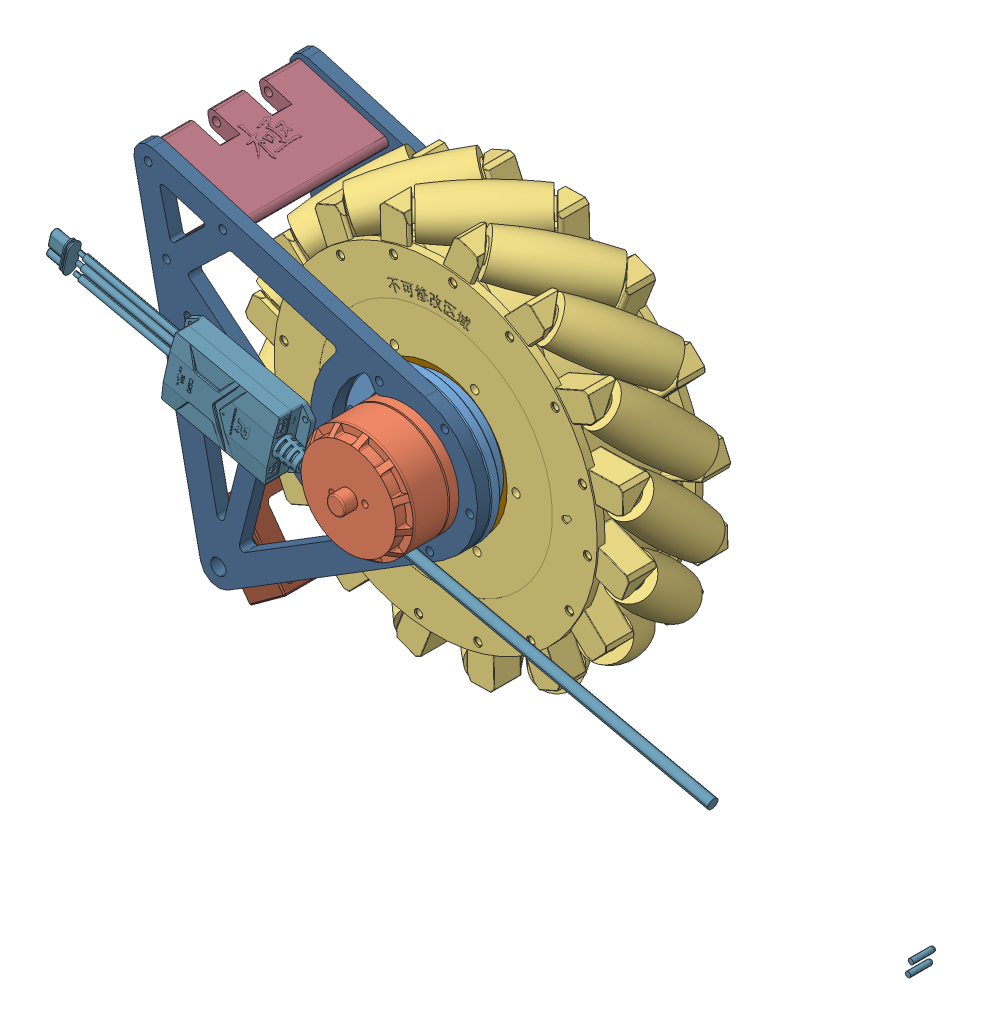
SolidWorks assembly 轮组2, configuration 默认. Lengths in mm.
Overall size (340.98 169.14 98.4).
20 component instances, 16 part files, 46 mates.
Components (placement in the parent):
- 轮组3508机加工件-1: 轮组3508机加工件 [默认] x (-0.923728 -0.383049 0) z (0 0 -1) size (56.5 56.5 41)
- RM3508直流无刷减速电机-1: RM3508直流无刷减速电机 [默认] at (-14.2303 -11.5943 46.941) x (-0.704187 0.710014 0) z (0 0 -1) size (42 44.97 98.4)
- HEXROLL_16-D154-2.0-1: HEXROLL_16-D154-2.0 [默认] at (0 0 -7.05) x (0.999858 0.01686 0) z (0 0 1) size (153.78 153.78 41)
- 轮组转动机加件-1: 轮组转动机加件 [默认] at (0 0 -42.1) x (0 0 -1) z (0.857472 0.51453 0) size (22 67 67)
- 轮组机加件-1: 轮组机加件 [默认] at (0 0 -18) x (0 0 1) z (0.01686 -0.999858 0) size (8 66 66)
- 胀紧套 ZZ21—10x20x13-1: 胀紧套 ZZ21—10x20x13 [默认] at (0 0 -47.8) x (-0.281461 -0.959573 0) z (0 0 -1) size (20 20 15.5)
- GB894．2-86轴用弹性挡圈B型25-1: GB894．2-86轴用弹性挡圈B型25 [默认] at (0 0 -62.2) x (-0.199141 -0.979971 0) z (0 0 1) size (28.2 30.93 1.2)
- 法兰轴承-1: 法兰轴承 [25*37*7-1.5] at (0 0 -61.6) x (0.478869 0.877886 0) z (0.877886 -0.478869 0) size (40 7 40)
- 深沟球轴承-1: 深沟球轴承 [45x58x7] at (0 0 -17) x (0.721643 -0.692266 0) z (-0.692266 -0.721643 0) size (58 7 58)
- 轮组转板-1: 轮组转板 [内侧板] at (-98.9523 52.4637 2.5) x (-0.97621 -0.216826 0) z (0 0 -1) size (120.47 137.51 5)
- 轮组转板-2: 轮组转板 [外侧板] at (-98.9523 52.4637 -57.6) x (-0.97621 -0.216826 0) z (0 0 -1) size (120.47 137.51 5)
- 轮组转点机加工件-1: 轮组转点机加工件 [默认] at (-71.8517 -69.551 -27.55) x (0 0 1) z (-0.808472 -0.588535 0) size (45 30 17)
- 轮组垫块-1: 轮组垫块 [默认] at (0 0 -61.6) x (0.97621 0.216826 0) z (0 0 1) size (56.5 56.5 1.5)
- 悬挂安装打印件-1: 悬挂安装打印件 [默认] at (-98.9523 52.4637 -27.6) x (0.722068 0.691822 0) z (0 0 1) size (37.46 32.98 55)
- C620无刷电机调速器-2: C620无刷电机调速器 [默认] at (-61.9578 -5.1134 10.4) x (-0.976343 0.216228 0) z (-0.216228 -0.976343 0) size (343.45 13.81 26.13)
- 深沟球轴承-2: 深沟球轴承 [6x13x5] at (-71.8517 -69.551 -50.05) x (-0.458973 -0.88845 0) z (-0.88845 0.458973 0) size (13 5 13)
- 深沟球轴承-3: 深沟球轴承 [6x13x5] at (-71.8517 -69.551 -10.05) x (0.999149 0.04124 0) z (0.04124 -0.999149 0) size (13 5 13)
- 推力球轴承-1: 推力球轴承 [F6-14M 6*14*5] at (-71.8517 -69.551 -5.05) x (-0.205581 -0.97864 0) z (-0.97864 0.205581 0) size (14 5 14)
- 推力球轴承-2: 推力球轴承 [F6-14M 6*14*5] at (-71.8517 -69.551 -55.05) x (0.195364 -0.980731 0) z (-0.980731 -0.195364 0) size (14 5 14)
- 轮组轴承压板-1: 轮组轴承压板 [默认] at (0 0 -63.6) x (0.97621 0.216826 0) z (0 0 1) size (56.5 56.5 2)
Mates (geometry in assembly coordinates):
- 同心1: concentric aligned: cylinder of 轮组3508机加工件-1 through (0 0 -4) axis (0 0 1) radius 28.25; cylinder of 轮组转板-1 through (0 0 0) axis (0 0 1) radius 28.25
- 重合2: coincident anti-aligned: plane of 轮组3508机加工件-1 through (0 0 0) normal (0 0 1); plane of 轮组转板-1 through (0 0 0) normal (0 0 -1)
- 同心2: concentric aligned: cylinder of 轮组3508机加工件-1 through (-9.7677 23.5551 -4) axis (0 0 -1) radius 1.65; cylinder of 轮组转板-1 through (-9.7677 23.5551 10) axis (0 0 -1) radius 1.525
- 同心3: concentric aligned: cylinder of 轮组3508机加工件-1 through (0 0 -41) axis (0 0 1) radius 21.05; cylinder of RM3508直流无刷减速电机-1 through (0 0 -29.5) axis (0 0 1) radius 21
- 重合3: coincident anti-aligned: plane of 轮组3508机加工件-1 through (0 0 -39.5) normal (0 0 1); plane of RM3508直流无刷减速电机-1 through (-4.9701 -12.0124 -39.5) normal (0 0 -1)
- 同心4: concentric anti-aligned: cylinder of 轮组3508机加工件-1 through (-16.1652 -6.7034 -46.5) axis (0 0 1) radius 2; cylinder of RM3508直流无刷减速电机-1 through (-16.1652 -6.7034 -39.5) axis (0 0 -1) radius 1.65
- 同心5: concentric anti-aligned: cylinder of 轮组3508机加工件-1 through (0 0 -17) axis (0 0 1) radius 22.5; cylinder of 深沟球轴承-1 through (0 0 -10) axis (0 0 -1) radius 29
- 同心6: concentric aligned: cylinder of 轮组机加件-1 through (0 0 -18) axis (0 0 -1) radius 29; cylinder of 深沟球轴承-1 through (0 0 -10) axis (0 0 -1) radius 29
- 重合4: coincident aligned: circle of 轮组机加件-1; plane of 深沟球轴承-1 through (0 0 -17) normal (0 0 -1)
- 重合5: coincident anti-aligned: plane of 轮组3508机加工件-1 through (0 0 -10) normal (0 0 -1); plane of 深沟球轴承-1 through (0 0 -10) normal (0 0 1)
- 同心7: concentric anti-aligned: cylinder of 轮组3508机加工件-1 through (0 0 -41) axis (0 0 1) radius 22.25; cylinder of HEXROLL_16-D154-2.0-1 through (0 0 -38) axis (0 0 -1) radius 27.55
- 重合6: coincident anti-aligned: plane of HEXROLL_16-D154-2.0-1 through (0 0 -10) normal (0 0 -1); plane of 轮组机加件-1 through (-32.9953 -0.5564 -10) normal (0 0 1)
- 同心8: concentric anti-aligned: cylinder of HEXROLL_16-D154-2.0-1 through (0 0 -38) axis (0 0 -1) radius 27.55; cylinder of 轮组转动机加件-1 through (0 0 -42.1) axis (0 0 1) radius 13.5
- 同心9: concentric aligned: cylinder of HEXROLL_16-D154-2.0-1 through (-15.0452 -27.1043 -14.5255) axis (0 0 1) radius 1.6; cylinder of 轮组机加件-1 through (-15.0452 -27.1043 -10) axis (0 0 1) radius 1.25
- 重合7: coincident anti-aligned: plane of HEXROLL_16-D154-2.0-1 through (0 0 -45.1) normal (0 0 1); plane of 轮组转动机加件-1 through (-14.1496 23.5805 -45.1) normal (0 0 -1)
- 同心10: concentric aligned: cylinder of HEXROLL_16-D154-2.0-1 through (-30.9956 -0.5227 -38) axis (0 0 -1) radius 1.6; cylinder of 轮组转动机加件-1 through (-30.9956 -0.5227 -45.1) axis (0 0 -1) radius 1.25
- 同心11: concentric aligned: cylinder of 轮组转动机加件-1 through (0 0 -54.6) axis (0 0 -1) radius 12.5; cylinder of 法兰轴承-1 through (0 0 -54.6) axis (0 0 -1) radius 12.5
- 重合8: coincident anti-aligned: plane of 轮组转动机加件-1 through (0 0 -54.6) normal (0 0 -1); plane of 法兰轴承-1 through (0 0 -54.6) normal (0 0 1)
- 同心12: concentric anti-aligned: cylinder of 轮组转动机加件-1 through (0 0 -42.1) axis (0 0 1) radius 11.6; cylinder of GB894．2-86轴用弹性挡圈B型25-1 through (0 0 -61.6) axis (0 0 -1) radius 14.1
- 重合9: coincident anti-aligned: plane of GB894．2-86轴用弹性挡圈B型25-1 through (-0.8134 0.1653 -61.6) normal (0 0 1); plane of 法兰轴承-1 through (0 0 -61.6) normal (0 0 -1)
- 同心13: concentric aligned: cylinder of 轮组转板-1 through (-71.8517 -69.551 0) axis (0 0 1) radius 3; cylinder of 轮组转板-2 through (-71.8517 -69.551 -60.1) axis (0 0 1) radius 3
- 同心14: concentric anti-aligned: cylinder of 法兰轴承-1 through (0 0 -54.6) axis (0 0 -1) radius 18.5; cylinder of 轮组转板-2 through (0 0 -60.1) axis (0 0 1) radius 18.5
- 重合10: coincident anti-aligned: plane of 法兰轴承-1 through (0 0 -60.1) normal (0 0 1); plane of 轮组转板-2 through (0 0 -60.1) normal (0 0 -1)
- 同心15: concentric anti-aligned: cylinder of 轮组转动机加件-1 through (0 0 -42.1) axis (0 0 1) radius 10; cylinder of 轮组垫块-1 through (0 0 -60.1) axis (0 0 -1) radius 20
- 重合11: coincident anti-aligned: plane of 轮组转板-2 through (0 0 -60.1) normal (0 0 -1); plane of 轮组垫块-1 through (0 0 -60.1) normal (0 0 1)
- 同心16: concentric anti-aligned: cylinder of 轮组转板-2 through (18.241 16.7281 -50.1) axis (0 0 -1) radius 1.525; cylinder of 轮组垫块-1 through (18.241 16.7281 -66.1255) axis (0 0 1) radius 1.6
- 同心17: concentric anti-aligned: cylinder of 轮组转动机加件-1 through (0 0 -42.1) axis (0 0 1) radius 10; cylinder of 轮组轴承压板-1 through (0 0 -61.6) axis (0 0 -1) radius 18.5
- 重合12: coincident anti-aligned: plane of 轮组垫块-1 through (0 0 -61.6) normal (0 0 -1); plane of 轮组轴承压板-1 through (0 0 -61.6) normal (0 0 1)
- 同心18: concentric anti-aligned: cylinder of 轮组转板-2 through (-5.3664 24.1612 -50.1) axis (0 0 -1) radius 1.525; cylinder of 轮组轴承压板-1 through (-5.3664 24.1612 -63.6) axis (0 0 1) radius 1.525
- 重合13: coincident anti-aligned: plane of 轮组转板-2 through (0 0 -55.1) normal (0 0 1); plane of 悬挂安装打印件-1 through (-98.9523 52.4637 -55.1) normal (0 0 -1)
- 同心19: concentric aligned: cylinder of 轮组转板-2 through (-70.1472 44.0811 -28.56) axis (0 0 -1) radius 1.525; cylinder of 悬挂安装打印件-1 through (-70.1472 44.0811 -0.1) axis (0 0 -1) radius 1.6
- 同心20: concentric anti-aligned: cylinder of 轮组转板-2 through (-98.9523 52.4637 -60.1) axis (0 0 1) radius 1.525; cylinder of 悬挂安装打印件-1 through (-98.9523 52.4637 -0.1) axis (0 0 -1) radius 1.6
- 同心21: concentric anti-aligned: cylinder of RM3508直流无刷减速电机-1 through (0 0 -66.8) axis (0 0 -1) radius 5; cylinder of 胀紧套 ZZ21—10x20x13-1 through (0 0 -60.8) axis (0 0 1) radius 10
- 距离2: distance = 6 mm aligned: plane of RM3508直流无刷减速电机-1 through (-1.9152 4.6186 -66.8) normal (0 0 -1); plane of 胀紧套 ZZ21—10x20x13-1 through (0 0 -60.8) normal (0 0 -1)
- 同心22: concentric anti-aligned: cylinder of 轮组转板-2 through (-71.8517 -69.551 -60.1) axis (0 0 1) radius 3; cylinder of 轮组转点机加工件-1 through (-71.8517 -69.551 -45.05) axis (0 0 -1) radius 6.5
- 重合14: coincident anti-aligned: plane of 轮组转板-1 through (0 0 5) normal (0 0 1); plane of C620无刷电机调速器-2 through (-60.298 -5.481 5) normal (0 0 -1)
- 同心23: concentric aligned: cylinder of 轮组转点机加工件-1 through (-71.8517 -69.551 -45.05) axis (0 0 -1) radius 6.5; cylinder of 深沟球轴承-2 through (-71.8517 -69.551 -45.05) axis (0 0 -1) radius 6.5
- 重合15: coincident anti-aligned: plane of 轮组转点机加工件-1 through (-71.8517 -69.551 -45.05) normal (0 0 -1); plane of 深沟球轴承-2 through (-71.8517 -69.551 -45.05) normal (0 0 1)
- 同心24: concentric anti-aligned: cylinder of 轮组转点机加工件-1 through (-71.8517 -69.551 -10.05) axis (0 0 1) radius 6.5; cylinder of 推力球轴承-1 through (-71.8517 -69.551 -0.05) axis (0 0 -1) radius 7
- 宽度1: width anti-aligned: plane of 轮组转板-2 through (0 0 -55.1) normal (0 0 1); plane of 轮组转板-1 through (0 0 0) normal (0 0 -1); plane of 轮组转点机加工件-1 through (-69.8957 -86.6806 -50.05) normal (0 0 -1); plane of 轮组转点机加工件-1 through (-69.8957 -86.6806 -5.05) normal (0 0 1)
- 同心25: concentric anti-aligned: cylinder of 轮组转点机加工件-1 through (-71.8517 -69.551 -63.05) axis (0 0 1) radius 4; cylinder of 深沟球轴承-3 through (-71.8517 -69.551 -5.05) axis (0 0 -1) radius 3
- 重合16: coincident anti-aligned: plane of 轮组转点机加工件-1 through (-71.8517 -69.551 -10.05) normal (0 0 1); plane of 深沟球轴承-3 through (-71.8517 -69.551 -10.05) normal (0 0 -1)
- 同心26: concentric aligned: cylinder of 深沟球轴承-3 through (-71.8517 -69.551 -5.05) axis (0 0 -1) radius 3; cylinder of 推力球轴承-1 through (-71.8517 -69.551 -0.05) axis (0 0 -1) radius 7
- 重合17: coincident anti-aligned: plane of 深沟球轴承-3 through (-71.8517 -69.551 -5.05) normal (0 0 1); plane of 推力球轴承-1 through (-71.8517 -69.551 -5.05) normal (0 0 -1)
- 同心27: concentric aligned: cylinder of 深沟球轴承-2 through (-71.8517 -69.551 -45.05) axis (0 0 -1) radius 3; cylinder of 推力球轴承-2 through (-71.8517 -69.551 -50.05) axis (0 0 -1) radius 7
- 重合18: coincident anti-aligned: plane of 深沟球轴承-2 through (-71.8517 -69.551 -50.05) normal (0 0 -1); plane of 推力球轴承-2 through (-71.8517 -69.551 -50.05) normal (0 0 1)
